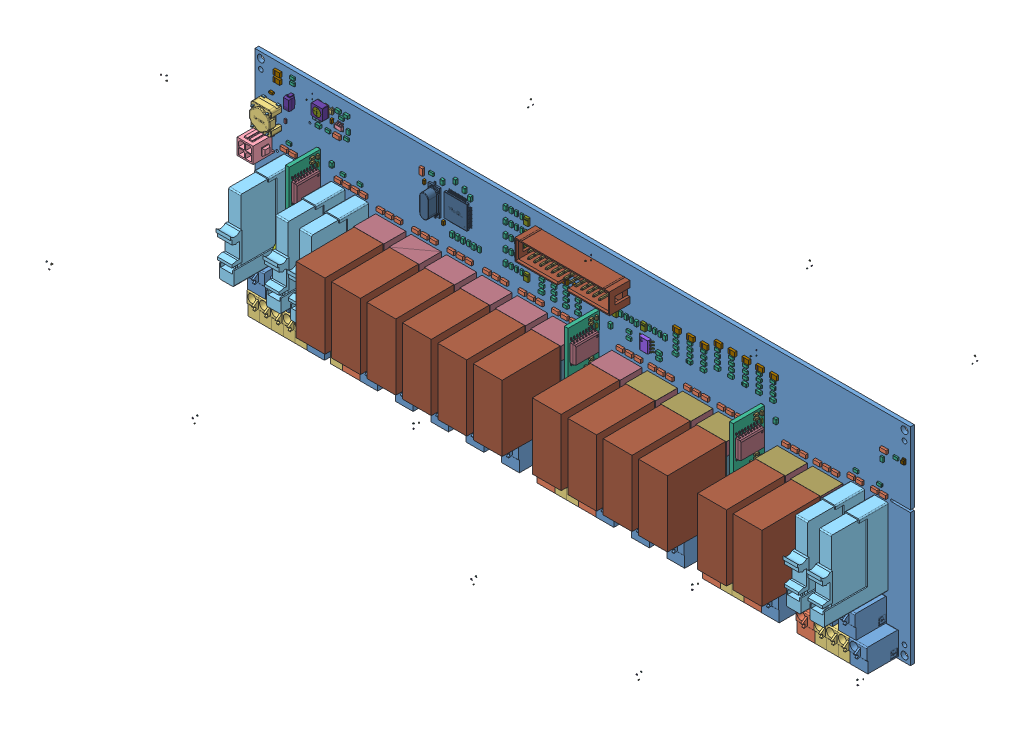
SolidWorks assembly _SC940D, configuration Default. Lengths in mm.
Overall size (350.55 148.8 148.76).
1323 component instances, 58 part files, 0 mates.
Components (placement in the parent):
- Board-1: Board [Default] at (0 0 -1.6703) size (281.94 89 1.67)
- D19-1: D19 [Default] at origin size (14.37 27.55 23.48)
  - SW3dPS-transistor_SOT233_4-1: SW3dPS-transistor_SOT233_4 [Default] at (10.8838 24.6832 -21.9) x (-1 0 0) z (0 1 0) size (2.9 1.1 1.6)
  - SW3dPS-transistor_SOT233_5-1: SW3dPS-transistor_SOT233_5 [Default] at (0.0109 0.0247 -0.0219) x (-1 0 0) z (0 1 0) size (2.18 2.18 2.18)
  - SW3dPS-transistor_SOT233_6-1: SW3dPS-transistor_SOT233_6 [Default] at (0 0 0) x (-1 0 0) z (0 1 0) size (2.18 2.18 2.18)
  - SW3dPS-transistor_SOT233_7-1: SW3dPS-transistor_SOT233_7 [Default] x (-1 0 0) z (0 1 0) size (2.18 2.18 2.18)
- U5-1: U5 [Default] at origin size (27.38 148.76 148.76)
  - SC943-0C_20-12-2012-1: SC943-0C_20-12-2012 [Default] at (142.3952 27.9566 3.7281) x (0 1 0.000663) z (1 0 0) size (148.66 148.66 27.38)
    - Board_1-1: Board_1 [Default] at (0 0 -1.6167) size (43.5 16.8 1.62)
    - R15-1: R15 [Default] at origin size (1.6 0.8 0.55)
      - RESC1608X84N_1-1: RESC1608X84N_1 [Default] at (-0.0001 1.9049 0) x (-1 0 0) z (0 1 0) size (1.6 0.55 0.8)
    - R11-1: R11 [Default] at origin size (2 1.2 0.7)
      - RESC2012X70N_1-1: RESC2012X70N_1 [Default] at (-3.6513 -0.4763 0) x (-1 0 0) z (0 1 0) size (2 0.7 1.2)
    - R7-1: R7 [Default] at origin size (2 1.2 0.7)
      - RESC2012X70N_1-1: RESC2012X70N_1 [Default] at (-5.2388 1.5874 0) x (-1 0 0) z (0 1 0) size (2 0.7 1.2)
    - D3-1: D3 [Default] at origin size (2.6 5.2 2.43)
      - SW3dPS-DO-214AC_SMA-1: SW3dPS-DO-214AC_SMA [Default] at (-1.4287 0.3175 -2.9167) x (1 0 0) z (0 0 -1) size (2.6 5.2 2.43)
    - T4-1: T4 [Default] at origin size (6.54 9.94 2.42)
      - SW3dPS-DPAK-1-1: SW3dPS-DPAK-1 [Default] at (10.9238 2.2758 -2.8167) x (1 0 0) z (0 1 0) size (6.54 2.42 9.94)
    - T3-1: T3 [Default] at origin size (6.54 9.94 2.42)
      - SW3dPS-DPAK-1-1: SW3dPS-DPAK-1 [Default] at (-10.3487 2.2758 -2.8167) x (1 0 0) z (0 1 0) size (6.54 2.42 9.94)
    - D5-1: D5 [Default] at origin size (2.6 5.2 2.43)
      - SW3dPS-DO-214AC_SMA-1: SW3dPS-DO-214AC_SMA [Default] at (2.0638 0.3175 -2.9167) x (1 0 0) z (0 0 -1) size (2.6 5.2 2.43)
    - D4-1: D4 [Default] at origin size (2.6 5.2 2.43)
      - SW3dPS-DO-214AC_SMA-1: SW3dPS-DO-214AC_SMA [Default] at (5.2388 0.3175 -2.9167) x (1 0 0) z (0 0 -1) size (2.6 5.2 2.43)
    - D2-1: D2 [Default] at origin size (2.6 5.2 2.43)
      - SW3dPS-DO-214AC_SMA-1: SW3dPS-DO-214AC_SMA [Default] at (-4.6037 0.3175 -2.9167) x (1 0 0) z (0 0 -1) size (2.6 5.2 2.43)
    - R25-1: R25 [Default] at origin size (3.2 1.6 0.84)
      - RESC3216X84N-1: RESC3216X84N [Default] at (-2.0851 5.5563 -1.6167) x (-1 0 0) z (0 -1 0) size (3.2 0.84 1.6)
    - R26-1: R26 [Default] at origin size (3.2 1.6 0.84)
      - RESC3216X84N-1: RESC3216X84N [Default] at (2.6989 5.5562 -1.6167) x (1 0 0) z (0 1 0) size (3.2 0.84 1.6)
    - C6-1: C6 [Default] at origin size (0.8 1.6 0.9)
      - User_Library-CAPC1608X09_1-1: User_Library-CAPC1608X09_1 [Default] at (10.0013 0.1587 0) x (0 -1 0) z (0 0 1) size (1.6 0.8 0.9)
    - C7-1: C7 [Default] at origin size (0.8 1.6 0.9)
      - User_Library-CAPC1608X09_1-1: User_Library-CAPC1608X09_1 [Default] at (27.7813 0.1587 0) x (0 -1 0) z (0 0 1) size (1.6 0.8 0.9)
    - C8-1: C8 [Default] at origin size (0.8 1.6 0.9)
      - User_Library-CAPC1608X09_1-1: User_Library-CAPC1608X09_1 [Default] at (26.1938 0.1587 0) x (0 -1 0) z (0 0 1) size (1.6 0.8 0.9)
    - C9-1: C9 [Default] at origin size (1.6 0.8 0.9)
      - User_Library-CAPC1608X09_1-1: User_Library-CAPC1608X09_1 [Default] at (7.7788 2.3813 0) size (1.6 0.8 0.9)
    - L1-1: L1 [Default] at origin size (1.6 0.8 0.9)
      - User_Library-CAPC1608X09_1-1: User_Library-CAPC1608X09_1 [Default] at (10.7949 -2.0638 0) x (-1 0 0) z (0 0 1) size (1.6 0.8 0.9)
    - L2-1: L2 [Default] at origin size (1.6 0.8 0.9)
      - User_Library-CAPC1608X09_1-1: User_Library-CAPC1608X09_1 [Default] at (27.1463 -2.2224 0) size (1.6 0.8 0.9)
    - L3-1: L3 [Default] at origin size (1.6 0.8 0.9)
      - User_Library-CAPC1608X09_1-1: User_Library-CAPC1608X09_1 [Default] at (10.7949 2.3812 0) x (-1 0 0) z (0 0 1) size (1.6 0.8 0.9)
    - U1-1: U1 [Default] at origin size (10.3 10.3 2.65)
      - SW3dPS-SOIC16-300-1: SW3dPS-SOIC16-300 [Default] at (19.685 3.9689 0) x (0 1 0) z (0 0 1) size (10.3 10.3 2.65)
    - R2-1: R2 [Default] at origin size (2 1.2 0.7)
      - RESC2012X70N_1-1: RESC2012X70N_1 [Default] at (-8.7312 1.9051 0) x (1 0 0) z (0 -1 0) size (2 0.7 1.2)
    - C4-1: C4 [Default] at origin size (0.8 1.6 0.9)
      - User_Library-CAPC1608X09_1-1: User_Library-CAPC1608X09_1 [Default] at (-13.0176 7.6201 0) x (0 1 0) z (0 0 1) size (1.6 0.8 0.9)
    - T6-1: T6 [Default] at origin size (36.29 81.18 23.48)
      - SW3dPS-transistor_SOT233-1: SW3dPS-transistor_SOT233 [Default] at (-33.4193 77.6987 -21.9) x (0 1 0) z (1 0 0) size (2.9 1.1 1.6)
      - SW3dPS-transistor_SOT233_1-1: SW3dPS-transistor_SOT233_1 [Default] at (-0.0334 0.0777 -0.0219) x (0 1 0) z (1 0 0) size (2.18 2.18 2.18)
      - SW3dPS-transistor_SOT233_2-1: SW3dPS-transistor_SOT233_2 [Default] at (0 0.0001 0) x (0 1 0) z (1 0 0) size (2.18 2.18 2.18)
      - SW3dPS-transistor_SOT233_3-1: SW3dPS-transistor_SOT233_3 [Default] x (0 1 0) z (1 0 0) size (2.18 2.18 2.18)
    - U2-1: U2 [Default] at origin size (6.2 5 1.75)
      - User_Library-SOIC-8-150-1: User_Library-SOIC-8-150 [Default] at (6.9849 6.3501 1) x (0 -1 0) z (-1 0 0) size (5 1.75 6.2)
        - User_Library-SOIC-8-150_pin_SOIC_SO-150_1_1-1: User_Library-SOIC-8-150_pin_SOIC_SO-150_1_1 [Default] at (0.6 0 -2) x (-1 0 0) z (0 0 -1) size (0.4 1.1 1.1)
        - User_Library-SOIC-8-150_pin_SOIC_SO-150_1_1-2: User_Library-SOIC-8-150_pin_SOIC_SO-150_1_1 [Default] at (-0.67 0 -2) x (-1 0 0) z (0 0 -1) size (0.4 1.1 1.1)
        - User_Library-SOIC-8-150_pin_SOIC_SO-150_1_1-3: User_Library-SOIC-8-150_pin_SOIC_SO-150_1_1 [Default] at (-1.94 0 2) size (0.4 1.1 1.1)
        - User_Library-SOIC-8-150_pin_SOIC_SO-150_1_1-4: User_Library-SOIC-8-150_pin_SOIC_SO-150_1_1 [Default] at (-0.67 0 2) size (0.4 1.1 1.1)
        - User_Library-SOIC-8-150_pin_SOIC_SO-150_1_1-5: User_Library-SOIC-8-150_pin_SOIC_SO-150_1_1 [Default] at (-1.94 0 -2) x (-1 0 0) z (0 0 -1) size (0.4 1.1 1.1)
        - User_Library-SOIC-8-150_pin_SOIC_SO-150_1_1-6: User_Library-SOIC-8-150_pin_SOIC_SO-150_1_1 [Default] at (1.87 0 2) size (0.4 1.1 1.1)
        - User_Library-SOIC-8-150_SOIC_150_SOIC_5X4_1_1-1: User_Library-SOIC-8-150_SOIC_150_SOIC_5X4_1_1 [Default] at origin size (5 1.5 4)
        - User_Library-SOIC-8-150_pin_SOIC_SO-150_1_1-7: User_Library-SOIC-8-150_pin_SOIC_SO-150_1_1 [Default] at (0.6 0 2) size (0.4 1.1 1.1)
        - User_Library-SOIC-8-150_pin_SOIC_SO-150_1_1-8: User_Library-SOIC-8-150_pin_SOIC_SO-150_1_1 [Default] at (1.87 0 -2) x (-1 0 0) z (0 0 -1) size (0.4 1.1 1.1)
    - R16-1: R16 [Default] at origin size (1.2 2 0.7)
      - RESC2012X70N_1-1: RESC2012X70N_1 [Default] at (-3.1751 7.3026 0) x (0 1 0) z (1 0 0) size (2 0.7 1.2)
    - R12-1: R12 [Default] at origin size (1.2 2 0.7)
      - RESC2012X70N_1-1: RESC2012X70N_1 [Default] at (2.2226 -1.2701 0) x (0 -1 0) z (-1 0 0) size (2 0.7 1.2)
    - R9-1: R9 [Default] at origin size (1.6 0.8 0.55)
      - RESC1608X84N_1-1: RESC1608X84N_1 [Default] at (1.5874 5.5562 0) x (-1 0 0) z (0 1 0) size (1.6 0.55 0.8)
    - R8-1: R8 [Default] at origin size (2 1.2 0.7)
      - RESC2012X70N_1-1: RESC2012X70N_1 [Default] at (5.0801 -1.9049 0) x (1 0 0) z (0 -1 0) size (2 0.7 1.2)
    - C5-1: C5 [Default] at origin size (0.8 1.6 0.9)
      - User_Library-CAPC1608X09_1-1: User_Library-CAPC1608X09_1 [Default] at (11.5888 0.1587 0) x (0 -1 0) z (0 0 1) size (1.6 0.8 0.9)
    - C3-1: C3 [Default] at origin size (0.8 1.6 0.9)
      - User_Library-CAPC1608X09_1-1: User_Library-CAPC1608X09_1 [Default] at (8.4138 0.1587 0) x (0 -1 0) z (0 0 1) size (1.6 0.8 0.9)
    - C2-1: C2 [Default] at origin size (0.8 1.6 0.9)
      - User_Library-CAPC1608X09_1-1: User_Library-CAPC1608X09_1 [Default] at (13.1763 0.1587 0) x (0 -1 0) z (0 0 1) size (1.6 0.8 0.9)
    - R17-1: R17 [Default] at origin size (0.8 1.6 0.55)
      - RESC1608X84N_1-1: RESC1608X84N_1 [Default] at (-1.2701 7.6201 0) x (0 1 0) z (1 0 0) size (1.6 0.55 0.8)
    - R18-1: R18 [Default] at origin size (1.6 0.8 0.55)
      - RESC1608X84N_1-1: RESC1608X84N_1 [Default] at (-6.9851 8.2549 0) x (-1 0 0) z (0 1 0) size (1.6 0.55 0.8)
    - T5-1: T5 [Default] at origin size (82.76 20.1 23.48)
      - SW3dPS-transistor_SOT233-1: SW3dPS-transistor_SOT233 [Default] at (-79.2862 -17.2268 -21.9) x (-1 0 0) z (0 1 0) size (2.9 1.1 1.6)
      - SW3dPS-transistor_SOT233_1-1: SW3dPS-transistor_SOT233_1 [Default] at (-0.0793 -0.0172 -0.0219) x (-1 0 0) z (0 1 0) size (2.18 2.18 2.18)
      - SW3dPS-transistor_SOT233_2-1: SW3dPS-transistor_SOT233_2 [Default] at (-0.0001 0 0) x (-1 0 0) z (0 1 0) size (2.18 2.18 2.18)
      - SW3dPS-transistor_SOT233_3-1: SW3dPS-transistor_SOT233_3 [Default] x (-1 0 0) z (0 1 0) size (2.18 2.18 2.18)
    - T7-1: T7 [Default] at origin size (73.54 29.78 23.48)
      - SW3dPS-transistor_SOT233-1: SW3dPS-transistor_SOT233 [Default] at (70.0609 26.9106 -21.9) x (1 0 0) z (0 -1 0) size (2.9 1.1 1.6)
      - SW3dPS-transistor_SOT233_1-1: SW3dPS-transistor_SOT233_1 [Default] at (0.0701 0.0269 -0.0219) x (1 0 0) z (0 -1 0) size (2.18 2.18 2.18)
      - SW3dPS-transistor_SOT233_2-1: SW3dPS-transistor_SOT233_2 [Default] at (0.0001 0 0) x (1 0 0) z (0 -1 0) size (2.18 2.18 2.18)
      - SW3dPS-transistor_SOT233_3-1: SW3dPS-transistor_SOT233_3 [Default] x (1 0 0) z (0 -1 0) size (2.18 2.18 2.18)
    - C1-1: C1 [Default] at origin size (1.6 0.8 0.9)
      - User_Library-CAPC1608X09_1-1: User_Library-CAPC1608X09_1 [Default] at (27.1462 -1.9049 -1.6167) x (-1 0 0) z (0 0 -1) size (1.6 0.8 0.9)
    - R19-1: R19 [Default] at origin size (1.6 0.8 0.55)
      - RESC1608X84N_1-1: RESC1608X84N_1 [Default] at (-10.7949 8.2551 0) x (1 0 0) z (0 -1 0) size (1.6 0.55 0.8)
    - R1-1: R1 [Default] at origin size (1.6 0.8 0.55)
      - RESC1608X84N_1-1: RESC1608X84N_1 [Default] at (24.1301 -2.2224 0) x (1 0 0) z (0 -1 0) size (1.6 0.55 0.8)
    - D1-1: D1 [Default] at origin size (80.06 27.08 23.48)
      - SW3dPS-transistor_SOT233-1: SW3dPS-transistor_SOT233 [Default] at (76.5874 24.2118 -21.9) x (1 0 0) z (0 -1 0) size (2.9 1.1 1.6)
      - SW3dPS-transistor_SOT233_1-1: SW3dPS-transistor_SOT233_1 [Default] at (0.0766 0.0242 -0.0219) x (1 0 0) z (0 -1 0) size (2.18 2.18 2.18)
      - SW3dPS-transistor_SOT233_2-1: SW3dPS-transistor_SOT233_2 [Default] at (0.0001 0 0) x (1 0 0) z (0 -1 0) size (2.18 2.18 2.18)
      - SW3dPS-transistor_SOT233_3-1: SW3dPS-transistor_SOT233_3 [Default] x (1 0 0) z (0 -1 0) size (2.18 2.18 2.18)
    - D6-1: D6 [Default] at origin size (13.75 77.05 23.48)
      - SW3dPS-transistor_SOT233-1: SW3dPS-transistor_SOT233 [Default] at (10.8768 -73.5712 -21.9) x (0 -1 0) z (-1 0 0) size (2.9 1.1 1.6)
      - SW3dPS-transistor_SOT233_1-1: SW3dPS-transistor_SOT233_1 [Default] at (0.0109 -0.0736 -0.0219) x (0 -1 0) z (-1 0 0) size (2.18 2.18 2.18)
      - SW3dPS-transistor_SOT233_2-1: SW3dPS-transistor_SOT233_2 [Default] at (0 -0.0001 0) x (0 -1 0) z (-1 0 0) size (2.18 2.18 2.18)
      - SW3dPS-transistor_SOT233_3-1: SW3dPS-transistor_SOT233_3 [Default] x (0 -1 0) z (-1 0 0) size (2.18 2.18 2.18)
    - D7-1: D7 [Default] at origin size (17.72 77.05 23.48)
      - SW3dPS-transistor_SOT233-1: SW3dPS-transistor_SOT233 [Default] at (14.8456 -73.5712 -21.9) x (0 -1 0) z (-1 0 0) size (2.9 1.1 1.6)
      - SW3dPS-transistor_SOT233_1-1: SW3dPS-transistor_SOT233_1 [Default] at (0.0148 -0.0736 -0.0219) x (0 -1 0) z (-1 0 0) size (2.18 2.18 2.18)
      - SW3dPS-transistor_SOT233_2-1: SW3dPS-transistor_SOT233_2 [Default] at (0 -0.0001 0) x (0 -1 0) z (-1 0 0) size (2.18 2.18 2.18)
      - SW3dPS-transistor_SOT233_3-1: SW3dPS-transistor_SOT233_3 [Default] x (0 -1 0) z (-1 0 0) size (2.18 2.18 2.18)
    - R3-1: R3 [Default] at origin size (2 1.2 0.7)
      - RESC2012X70N_1-1: RESC2012X70N_1 [Default] at (-12.2237 1.9051 0) x (1 0 0) z (0 -1 0) size (2 0.7 1.2)
- L3_1-1: L3_1 [Default] at origin size (8.76 10 6)
  - STEP-744272102-rev1_RGB8421504-1: STEP-744272102-rev1_RGB8421504 [Default] at (1.7783 60.1986 0.3127) x (-1 0 0) z (0 0 1) size (8.76 10 6)
    - Base_5-1: Base_5 [Default] at origin size (5 6.5 2.6)
    - Base_6-1: Base_6 [Default] at origin size (8.76 10 5.3)
    - Base_1-1: Base_1 [Default] at origin size (3.01 7.71 4.33)
    - Contact-1: Contact [Default] at (-3.11 -3.66 -0.3) x (-1 0 0) z (0 0 -1) size (1.2 1.83 6)
    - Contact-2: Contact [Default] at (3.11 -3.66 -0.3) x (-1 0 0) z (0 0 -1) size (1.2 1.83 6)
    - Contact-3: Contact [Default] at (-3.11 3.66 -0.3) x (1 0 0) z (0 0 -1) size (1.2 1.83 6)
    - Contact-4: Contact [Default] at (3.11 3.66 -0.3) x (1 0 0) z (0 0 -1) size (1.2 1.83 6)
- C39-1: C39 [Default] at origin size (2 1.25 1)
  - User_Library-CAPC2013X10-1: User_Library-CAPC2013X10 [Default] at (168.5924 52.2287 0) x (-1 0 0) z (0 0 1) size (2 1.25 1)
- C38-1: C38 [Default] at origin size (2 1.25 1)
  - User_Library-CAPC2013X10-1: User_Library-CAPC2013X10 [Default] at (168.5926 54.2926 0) x (1 0 0) z (0 0 1) size (2 1.25 1)
- VR1-1: VR1 [Default] at origin size (3.59 9 34)
  - WE-VD_7_mm-1: WE-VD_7_mm [Default] at (15.5576 20.1613 9) x (0 1 0) z (0 0 1) size (9 3.59 34)
- D38-1: D38 [Default] at origin size (2.9 1.9 0.99)
  - 905269800-1: 905269800 [Default] at (187.579 66.802 0.95) size (0.25 1.78 0.04)
    - Extruded-1: Extruded [Default] at origin size (0.25 1.78 0.04)
  - 905269392-1: 905269392 [Default] at (188.214 66.802 0) size (2.9 1.9 0.98)
    - Extruded_1-1: Extruded_1 [Default] at origin size (2.9 1.9 0.98)
- U4-1: U4 [Default] at origin size (12.02 12.02 1.1)
  - User_Library-TQFP64-1: User_Library-TQFP64 [Default] at (81.6561 63.8895 0) x (-1 0 0) z (0 0 1) size (12.02 12.02 1.1)
- K13-1: K13 [Default] at origin size (13 30.3 34.5)
  - relais_40_61_8_006_0000-1: relais_40_61_8_006_0000 [Default] at (200.025 15.6766 9.5) x (0 1 0) z (1 0 0) size (29 30 12.4)
  - 1151724792-1: 1151724792 [Default] at (200.025 21.78 0) size (13 14.8 9.5)
    - Extruded_2-1: Extruded_2 [Default] at origin size (13 14.8 9.5)
  - 1151724928-1: 1151724928 [Default] at (200.025 41.93 0) size (13 5.5 9.5)
    - Extruded_3-1: Extruded_3 [Default] at origin size (13 5.5 9.5)
  - 1151725064-1: 1151725064 [Default] at (200.025 34.18 5) size (13 10 4.5)
    - Extruded_4-1: Extruded_4 [Default] at origin size (13 10 4.5)
- SUP_K13-1: SUP_K13 [Default] at origin size (13 30.3 9.5)
  - 1151724792-1: 1151724792 [Default] at (200.025 37.325 0) size (13 14.8 9.5)
    - Extruded_2-1: Extruded_2 [Default] at origin size (13 14.8 9.5)
  - 1151725064-1: 1151725064 [Default] at (200.025 24.925 5) size (13 10 4.5)
    - Extruded_4-1: Extruded_4 [Default] at origin size (13 10 4.5)
  - 1151724928-1: 1151724928 [Default] at (200.025 17.175 0) size (13 5.5 9.5)
    - Extruded_3-1: Extruded_3 [Default] at origin size (13 5.5 9.5)
- SUP_K12-1: SUP_K12 [Default] at origin size (13 30.3 9.5)
  - 1151724792-1: 1151724792 [Default] at (184.785 37.325 0) size (13 14.8 9.5)
    - Extruded_2-1: Extruded_2 [Default] at origin size (13 14.8 9.5)
  - 1151725064-1: 1151725064 [Default] at (184.785 24.925 5) size (13 10 4.5)
    - Extruded_4-1: Extruded_4 [Default] at origin size (13 10 4.5)
  - 1151724928-1: 1151724928 [Default] at (184.785 17.175 0) size (13 5.5 9.5)
    - Extruded_3-1: Extruded_3 [Default] at origin size (13 5.5 9.5)
- K12-1: K12 [Default] at origin size (13 30.3 34.5)
  - relais_40_61_8_006_0000-1: relais_40_61_8_006_0000 [Default] at (184.785 15.6766 9.5) x (0 1 0) z (1 0 0) size (29 30 12.4)
  - 1151724792-1: 1151724792 [Default] at (184.785 21.78 0) size (13 14.8 9.5)
    - Extruded_2-1: Extruded_2 [Default] at origin size (13 14.8 9.5)
  - 1151724928-1: 1151724928 [Default] at (184.785 41.93 0) size (13 5.5 9.5)
    - Extruded_3-1: Extruded_3 [Default] at origin size (13 5.5 9.5)
  - 1151725064-1: 1151725064 [Default] at (184.785 34.18 5) size (13 10 4.5)
    - Extruded_4-1: Extruded_4 [Default] at origin size (13 10 4.5)
- C34-1: C34 [Default] at origin size (1.25 2 1)
  - User_Library-CAPC2013X10-1: User_Library-CAPC2013X10 [Default] at (218.8159 54.1717 0) x (0 -1 0) z (0 0 1) size (2 1.25 1)
- C27-1: C27 [Default] at origin size (1.25 2 1)
  - User_Library-CAPC2013X10-1: User_Library-CAPC2013X10 [Default] at (147.6959 54.1717 0) x (0 -1 0) z (0 0 1) size (2 1.25 1)
- C5_1-1: C5_1 [Default] at origin size (1.25 2 1)
  - User_Library-CAPC2013X10-1: User_Library-CAPC2013X10 [Default] at (27.8194 54.1717 0) x (0 -1 0) z (0 0 1) size (2 1.25 1)
- VR2-1: VR2 [Default] at origin size (3.59 9 34)
  - WE-VD_7_mm-1: WE-VD_7_mm [Default] at (133.9849 8.3979 9) x (0 -1 0) z (0 0 1) size (9 3.59 34)
- D28-1: D28 [Default] at origin size (1.9 2.9 0.99)
  - 1151710512-1: 1151710512 [Default] at (162.052 61.595 0.95) size (1.78 0.25 0.04)
    - Extruded_5-1: Extruded_5 [Default] at origin size (1.78 0.25 0.04)
  - 1151710376-1: 1151710376 [Default] at (162.052 60.96 0) size (1.9 2.9 0.98)
    - Extruded_6-1: Extruded_6 [Default] at origin size (1.9 2.9 0.98)
- VR3-1: VR3 [Default] at origin size (3.59 9 34)
  - WE-VD_7_mm-1: WE-VD_7_mm [Default] at (205.1049 8.3979 9) x (0 -1 0) z (0 0 1) size (9 3.59 34)
- D2_1-1: D2_1 [Default] at origin size (2.9 1.9 0.99)
  - 905269800-1: 905269800 [Default] at (3.8418 73.803 0.95) size (0.25 1.78 0.04)
    - Extruded-1: Extruded [Default] at origin size (0.25 1.78 0.04)
  - 905269392-1: 905269392 [Default] at (4.4767 73.803 0) size (2.9 1.9 0.98)
    - Extruded_1-1: Extruded_1 [Default] at origin size (2.9 1.9 0.98)
- D1_1-1: D1_1 [Default] at origin size (2.9 1.9 0.99)
  - 905269800-1: 905269800 [Default] at (3.8418 76.5017 0.95) size (0.25 1.78 0.04)
    - Extruded-1: Extruded [Default] at origin size (0.25 1.78 0.04)
  - 905269392-1: 905269392 [Default] at (4.4767 76.5017 0) size (2.9 1.9 0.98)
    - Extruded_1-1: Extruded_1 [Default] at origin size (2.9 1.9 0.98)
- D41-1: D41 [Default] at origin size (2.9 1.9 0.99)
  - 905269800-1: 905269800 [Default] at (193.548 70.358 0.95) size (0.25 1.78 0.04)
    - Extruded-1: Extruded [Default] at origin size (0.25 1.78 0.04)
  - 905269392-1: 905269392 [Default] at (194.183 70.358 0) size (2.9 1.9 0.98)
    - Extruded_1-1: Extruded_1 [Default] at origin size (2.9 1.9 0.98)
- D40-1: D40 [Default] at origin size (2.9 1.9 0.99)
  - 905269800-1: 905269800 [Default] at (199.517 70.358 0.95) size (0.25 1.78 0.04)
    - Extruded-1: Extruded [Default] at origin size (0.25 1.78 0.04)
  - 905269392-1: 905269392 [Default] at (200.152 70.358 0) size (2.9 1.9 0.98)
    - Extruded_1-1: Extruded_1 [Default] at origin size (2.9 1.9 0.98)
- D36-1: D36 [Default] at origin size (2.9 1.9 0.99)
  - 905269800-1: 905269800 [Default] at (205.486 70.358 0.95) size (0.25 1.78 0.04)
    - Extruded-1: Extruded [Default] at origin size (0.25 1.78 0.04)
  - 905269392-1: 905269392 [Default] at (206.121 70.358 0) size (2.9 1.9 0.98)
    - Extruded_1-1: Extruded_1 [Default] at origin size (2.9 1.9 0.98)
- D35-1: D35 [Default] at origin size (2.9 1.9 0.99)
  - 905269800-1: 905269800 [Default] at (181.61 66.802 0.95) size (0.25 1.78 0.04)
    - Extruded-1: Extruded [Default] at origin size (0.25 1.78 0.04)
  - 905269392-1: 905269392 [Default] at (182.245 66.802 0) size (2.9 1.9 0.98)
    - Extruded_1-1: Extruded_1 [Default] at origin size (2.9 1.9 0.98)
- D33-1: D33 [Default] at origin size (2.9 1.9 0.99)
  - 905269800-1: 905269800 [Default] at (211.455 70.358 0.95) size (0.25 1.78 0.04)
    - Extruded-1: Extruded [Default] at origin size (0.25 1.78 0.04)
  - 905269392-1: 905269392 [Default] at (212.09 70.358 0) size (2.9 1.9 0.98)
    - Extruded_1-1: Extruded_1 [Default] at origin size (2.9 1.9 0.98)
- D32-1: D32 [Default] at origin size (2.9 1.9 0.99)
  - 905269800-1: 905269800 [Default] at (217.424 70.358 0.95) size (0.25 1.78 0.04)
    - Extruded-1: Extruded [Default] at origin size (0.25 1.78 0.04)
  - 905269392-1: 905269392 [Default] at (218.059 70.358 0) size (2.9 1.9 0.98)
    - Extruded_1-1: Extruded_1 [Default] at origin size (2.9 1.9 0.98)
- D30-1: D30 [Default] at origin size (2.9 1.9 0.99)
  - 905269800-1: 905269800 [Default] at (175.641 66.802 0.95) size (0.25 1.78 0.04)
    - Extruded-1: Extruded [Default] at origin size (0.25 1.78 0.04)
  - 905269392-1: 905269392 [Default] at (176.276 66.802 0) size (2.9 1.9 0.98)
    - Extruded_1-1: Extruded_1 [Default] at origin size (2.9 1.9 0.98)
- D26-1: D26 [Default] at origin size (1.9 2.9 0.99)
  - 1151710512-1: 1151710512 [Default] at (149.733 60.706 0.95) size (1.78 0.25 0.04)
    - Extruded_5-1: Extruded_5 [Default] at origin size (1.78 0.25 0.04)
  - 1151710376-1: 1151710376 [Default] at (149.733 60.071 0) size (1.9 2.9 0.98)
    - Extruded_6-1: Extruded_6 [Default] at origin size (1.9 2.9 0.98)
- D22-1: D22 [Default] at origin size (1.9 2.9 0.99)
  - 1151710512-1: 1151710512 [Default] at (137.414 60.706 0.95) size (1.78 0.25 0.04)
    - Extruded_5-1: Extruded_5 [Default] at origin size (1.78 0.25 0.04)
  - 1151710376-1: 1151710376 [Default] at (137.414 60.071 0) size (1.9 2.9 0.98)
    - Extruded_6-1: Extruded_6 [Default] at origin size (1.9 2.9 0.98)
- D20-1: D20 [Default] at origin size (2.9 1.9 0.99)
  - 905269800-1: 905269800 [Default] at (133.858 60.96 0.95) size (0.25 1.78 0.04)
    - Extruded-1: Extruded [Default] at origin size (0.25 1.78 0.04)
  - 905269392-1: 905269392 [Default] at (133.223 60.96 0) size (2.9 1.9 0.98)
    - Extruded_1-1: Extruded_1 [Default] at origin size (2.9 1.9 0.98)
- D17-1: D17 [Default] at origin size (2.9 1.9 0.99)
  - 905269800-1: 905269800 [Default] at (123.444 60.96 0.95) size (0.25 1.78 0.04)
    - Extruded-1: Extruded [Default] at origin size (0.25 1.78 0.04)
  - 905269392-1: 905269392 [Default] at (122.809 60.96 0) size (2.9 1.9 0.98)
    - Extruded_1-1: Extruded_1 [Default] at origin size (2.9 1.9 0.98)
- D14-1: D14 [Default] at origin size (2.9 1.9 0.99)
  - 905269800-1: 905269800 [Default] at (128.651 60.96 0.95) size (0.25 1.78 0.04)
    - Extruded-1: Extruded [Default] at origin size (0.25 1.78 0.04)
  - 905269392-1: 905269392 [Default] at (128.016 60.96 0) size (2.9 1.9 0.98)
    - Extruded_1-1: Extruded_1 [Default] at origin size (2.9 1.9 0.98)
- D12-1: D12 [Default] at origin size (2.9 1.9 0.99)
  - 905269800-1: 905269800 [Default] at (118.237 60.96 0.95) size (0.25 1.78 0.04)
    - Extruded-1: Extruded [Default] at origin size (0.25 1.78 0.04)
  - 905269392-1: 905269392 [Default] at (117.602 60.96 0) size (2.9 1.9 0.98)
    - Extruded_1-1: Extruded_1 [Default] at origin size (2.9 1.9 0.98)
- D21-1: D21 [Default] at origin size (1.9 2.9 0.99)
  - 1151710512-1: 1151710512 [Default] at (111.76 60.071 0.95) size (1.78 0.25 0.04)
    - Extruded_5-1: Extruded_5 [Default] at origin size (1.78 0.25 0.04)
  - 1151710376-1: 1151710376 [Default] at (111.76 59.436 0) size (1.9 2.9 0.98)
    - Extruded_6-1: Extruded_6 [Default] at origin size (1.9 2.9 0.98)
- D18-1: D18 [Default] at origin size (1.9 2.9 0.99)
  - 1151710512-1: 1151710512 [Default] at (111.76 54.864 0.95) size (1.78 0.25 0.04)
    - Extruded_5-1: Extruded_5 [Default] at origin size (1.78 0.25 0.04)
  - 1151710376-1: 1151710376 [Default] at (111.76 54.229 0) size (1.9 2.9 0.98)
    - Extruded_6-1: Extruded_6 [Default] at origin size (1.9 2.9 0.98)
- D16-1: D16 [Default] at origin size (1.9 2.9 0.99)
  - 1151710512-1: 1151710512 [Default] at (111.76 75.692 0.95) size (1.78 0.25 0.04)
    - Extruded_5-1: Extruded_5 [Default] at origin size (1.78 0.25 0.04)
  - 1151710376-1: 1151710376 [Default] at (111.76 75.057 0) size (1.9 2.9 0.98)
    - Extruded_6-1: Extruded_6 [Default] at origin size (1.9 2.9 0.98)
- D13-1: D13 [Default] at origin size (1.9 2.9 0.99)
  - 1151710512-1: 1151710512 [Default] at (111.76 65.278 0.95) size (1.78 0.25 0.04)
    - Extruded_5-1: Extruded_5 [Default] at origin size (1.78 0.25 0.04)
  - 1151710376-1: 1151710376 [Default] at (111.76 64.643 0) size (1.9 2.9 0.98)
    - Extruded_6-1: Extruded_6 [Default] at origin size (1.9 2.9 0.98)
- D10-1: D10 [Default] at origin size (1.9 2.9 0.99)
  - 1151710512-1: 1151710512 [Default] at (111.76 70.485 0.95) size (1.78 0.25 0.04)
    - Extruded_5-1: Extruded_5 [Default] at origin size (1.78 0.25 0.04)
  - 1151710376-1: 1151710376 [Default] at (111.76 69.85 0) size (1.9 2.9 0.98)
    - Extruded_6-1: Extruded_6 [Default] at origin size (1.9 2.9 0.98)
- C6_1-1: C6_1 [Default] at origin size (1.25 2 1)
  - User_Library-CAPC2013X10-1: User_Library-CAPC2013X10 [Default] at (102.616 70.3579 0) x (0 -1 0) z (0 0 1) size (2 1.25 1)
- C8_1-1: C8_1 [Default] at origin size (1.25 2 1)
  - User_Library-CAPC2013X10-1: User_Library-CAPC2013X10 [Default] at (102.616 65.1509 0) x (0 -1 0) z (0 0 1) size (2 1.25 1)
- C10-1: C10 [Default] at origin size (1.25 2 1)
  - User_Library-CAPC2013X10-1: User_Library-CAPC2013X10 [Default] at (102.616 75.5649 0) x (0 -1 0) z (0 0 1) size (2 1.25 1)
- C12-1: C12 [Default] at origin size (1.25 2 1)
  - User_Library-CAPC2013X10-1: User_Library-CAPC2013X10 [Default] at (102.616 54.7369 0) x (0 -1 0) z (0 0 1) size (2 1.25 1)
- C11-1: C11 [Default] at origin size (2 1.25 1)
  - User_Library-CAPC2013X10-1: User_Library-CAPC2013X10 [Default] at (123.3169 51.816 0) x (-1 0 0) z (0 0 1) size (2 1.25 1)
- C28-1: C28 [Default] at origin size (1.25 2 1)
  - User_Library-CAPC2013X10-1: User_Library-CAPC2013X10 [Default] at (171.196 61.4679 0) x (0 -1 0) z (0 0 1) size (2 1.25 1)
- C14-1: C14 [Default] at origin size (1.25 2 1)
  - User_Library-CAPC2013X10-1: User_Library-CAPC2013X10 [Default] at (102.616 59.9439 0) x (0 -1 0) z (0 0 1) size (2 1.25 1)
- C7_1-1: C7_1 [Default] at origin size (2 1.25 1)
  - User_Library-CAPC2013X10-1: User_Library-CAPC2013X10 [Default] at (118.1099 51.816 0) x (-1 0 0) z (0 0 1) size (2 1.25 1)
- C9_1-1: C9_1 [Default] at origin size (2 1.25 1)
  - User_Library-CAPC2013X10-1: User_Library-CAPC2013X10 [Default] at (128.5239 51.816 0) x (-1 0 0) z (0 0 1) size (2 1.25 1)
- C13-1: C13 [Default] at origin size (2 1.25 1)
  - User_Library-CAPC2013X10-1: User_Library-CAPC2013X10 [Default] at (133.7309 51.816 0) x (-1 0 0) z (0 0 1) size (2 1.25 1)
- C15-1: C15 [Default] at origin size (1.25 2 1)
  - User_Library-CAPC2013X10-1: User_Library-CAPC2013X10 [Default] at (146.558 60.5789 0) x (0 -1 0) z (0 0 1) size (2 1.25 1)
- C26-1: C26 [Default] at origin size (1.25 2 1)
  - User_Library-CAPC2013X10-1: User_Library-CAPC2013X10 [Default] at (158.877 60.5789 0) x (0 -1 0) z (0 0 1) size (2 1.25 1)
- C29-1: C29 [Default] at origin size (2 1.25 1)
  - User_Library-CAPC2013X10-1: User_Library-CAPC2013X10 [Default] at (175.7681 57.658 0) x (1 0 0) z (0 0 1) size (2 1.25 1)
- C30-1: C30 [Default] at origin size (2 1.25 1)
  - User_Library-CAPC2013X10-1: User_Library-CAPC2013X10 [Default] at (217.5511 61.214 0) x (1 0 0) z (0 0 1) size (2 1.25 1)
- C31-1: C31 [Default] at origin size (2 1.25 1)
  - User_Library-CAPC2013X10-1: User_Library-CAPC2013X10 [Default] at (211.5821 61.214 0) x (1 0 0) z (0 0 1) size (2 1.25 1)
- C32-1: C32 [Default] at origin size (2 1.25 1)
  - User_Library-CAPC2013X10-1: User_Library-CAPC2013X10 [Default] at (181.7371 57.658 0) x (1 0 0) z (0 0 1) size (2 1.25 1)
- C33-1: C33 [Default] at origin size (2 1.25 1)
  - User_Library-CAPC2013X10-1: User_Library-CAPC2013X10 [Default] at (205.6131 61.214 0) x (1 0 0) z (0 0 1) size (2 1.25 1)
- C35-1: C35 [Default] at origin size (2 1.25 1)
  - User_Library-CAPC2013X10-1: User_Library-CAPC2013X10 [Default] at (187.7061 57.642 0) x (1 0 0) z (0 0 1) size (2 1.25 1)
- C36-1: C36 [Default] at origin size (2 1.25 1)
  - User_Library-CAPC2013X10-1: User_Library-CAPC2013X10 [Default] at (199.6441 61.214 0) x (1 0 0) z (0 0 1) size (2 1.25 1)
- C37-1: C37 [Default] at origin size (2 1.25 1)
  - User_Library-CAPC2013X10-1: User_Library-CAPC2013X10 [Default] at (193.6751 61.214 0) x (1 0 0) z (0 0 1) size (2 1.25 1)
- C19-1: C19 [Default] at origin size (1.25 2 1)
  - User_Library-CAPC2013X10-1: User_Library-CAPC2013X10 [Default] at (87.3799 71.3594 0) x (0 -1 0) z (0 0 1) size (2 1.25 1)
- C20-1: C20 [Default] at origin size (1.25 2 1)
  - User_Library-CAPC2013X10-1: User_Library-CAPC2013X10 [Default] at (75.4736 71.5181 0) x (0 -1 0) z (0 0 1) size (2 1.25 1)
- C18-1: C18 [Default] at origin size (1.25 2 1)
  - User_Library-CAPC2013X10-1: User_Library-CAPC2013X10 [Default] at (81.0298 74.5344 0) x (0 -1 0) z (0 0 1) size (2 1.25 1)
- C24-1: C24 [Default] at origin size (1.25 2 1)
  - User_Library-CAPC2013X10-1: User_Library-CAPC2013X10 [Default] at (81.9823 54.0559 0) x (0 1 0) z (0 0 1) size (2 1.25 1)
- C17-1: C17 [Default] at origin size (1.25 2 1)
  - User_Library-CAPC2013X10-1: User_Library-CAPC2013X10 [Default] at (84.9986 73.2644 0) x (0 -1 0) z (0 0 1) size (2 1.25 1)
- C16-1: C16 [Default] at origin size (1.25 2 1)
  - User_Library-CAPC2013X10-1: User_Library-CAPC2013X10 [Default] at (79.629 53.9749 0) x (0 -1 0) z (0 0 1) size (2 1.25 1)
- C23-1: C23 [Default] at origin size (1.25 2 1)
  - User_Library-CAPC2013X10-1: User_Library-CAPC2013X10 [Default] at (88.9 54.1021 0) x (0 1 0) z (0 0 1) size (2 1.25 1)
- C25-1: C25 [Default] at origin size (1.25 2 1)
  - User_Library-CAPC2013X10-1: User_Library-CAPC2013X10 [Default] at (84.328 54.1021 0) x (0 1 0) z (0 0 1) size (2 1.25 1)
- D3_1-1: D3_1 [Default] at origin size (2.6 5.25 2.98)
  - SW3dPS-DO-214BA-1: SW3dPS-DO-214BA [Default] at (10.541 69.0721 1.9) x (-1 0 0) z (0 0 1) size (2.6 5.25 2.98)
- DL1-1: DL1 [Default] at origin size (1.27 2.03 1.11)
  - SW3dPS-led805-1: SW3dPS-led805 [Default] at (273.6851 66.3799 0) x (1 0 0) z (0 -1 0) size (1.27 1.11 2.03)
- J42-1: J42 [Default] at origin size (7.62 10 19.2)
  - 1790487-1: 1790487 [Default] at (129.945 -5.67 -10.6) x (0 1 0) z (1 0 0) size (10 19.2 7.62)
    - ffkdsa1-v2-7.62-1: ffkdsa1-v2-7.62 [Default] at (-15.6914 -27.508 9.12) x (0 -1 0) z (0 0 1) size (19.2 10 7.62)
- J47-1: J47 [Default] at origin size (7.62 10 19.2)
  - 1790487-1: 1790487 [Default] at (140.105 -5.67 -10.6) x (0 1 0) z (1 0 0) size (10 19.2 7.62)
    - ffkdsa1-v2-7.62-1: ffkdsa1-v2-7.62 [Default] at (-15.6914 -27.508 9.12) x (0 -1 0) z (0 0 1) size (19.2 10 7.62)
- J66-1: J66 [Default] at origin size (7.62 10 19.2)
  - 1790487-1: 1790487 [Default] at (211.225 -5.67 -10.6) x (0 1 0) z (1 0 0) size (10 19.2 7.62)
    - ffkdsa1-v2-7.62-1: ffkdsa1-v2-7.62 [Default] at (-15.6914 -27.508 9.12) x (0 -1 0) z (0 0 1) size (19.2 10 7.62)
- J74-1: J74 [Default] at origin size (7.62 10 19.2)
  - 1790487-1: 1790487 [Default] at (241.705 -5.67 -10.6) x (0 1 0) z (1 0 0) size (10 19.2 7.62)
    - ffkdsa1-v2-7.62-1: ffkdsa1-v2-7.62 [Default] at (-15.6914 -27.508 9.12) x (0 -1 0) z (0 0 1) size (19.2 10 7.62)
- J79-1: J79 [Default] at origin size (7.62 10 19.2)
  - 1790487-1: 1790487 [Default] at (251.865 -5.67 -10.6) x (0 1 0) z (1 0 0) size (10 19.2 7.62)
    - ffkdsa1-v2-7.62-1: ffkdsa1-v2-7.62 [Default] at (-15.6914 -27.508 9.12) x (0 -1 0) z (0 0 1) size (19.2 10 7.62)
- J31-1: J31 [Default] at origin size (7.62 10 19.2)
  - 1790487-1: 1790487 [Default] at (76.605 -15.67 -10.6) x (0 1 0) z (1 0 0) size (10 19.2 7.62)
    - ffkdsa1-v2-7.62-1: ffkdsa1-v2-7.62 [Default] at (-15.6914 -27.508 9.12) x (0 -1 0) z (0 0 1) size (19.2 10 7.62)
- J34-1: J34 [Default] at origin size (7.62 10 19.2)
  - 1790487-1: 1790487 [Default] at (91.845 -15.67 -10.6) x (0 1 0) z (1 0 0) size (10 19.2 7.62)
    - ffkdsa1-v2-7.62-1: ffkdsa1-v2-7.62 [Default] at (-15.6914 -27.508 9.12) x (0 -1 0) z (0 0 1) size (19.2 10 7.62)
- J37-1: J37 [Default] at origin size (7.62 10 19.2)
  - 1790487-1: 1790487 [Default] at (107.085 -15.67 -10.6) x (0 1 0) z (1 0 0) size (10 19.2 7.62)
    - ffkdsa1-v2-7.62-1: ffkdsa1-v2-7.62 [Default] at (-15.6914 -27.508 9.12) x (0 -1 0) z (0 0 1) size (19.2 10 7.62)
- J40-1: J40 [Default] at origin size (9.42 10 19.2)
  - 1790377-1: 1790377 [Default] at (136.5251 -7.6199 0) x (0 1 0) z (1 0 0) size (10 19.2 9.42)
    - ffkdsa-v2-7.62-1: ffkdsa-v2-7.62 [Default] at (-23.7414 -38.158 -5.08) x (0 -1 0) z (0 0 1) size (19.2 10 9.42)
- J43-1: J43 [Default] at origin size (6.88 10 19.2)
  - 1790348-1: 1790348 [Default] at (141.6051 -7.6199 0) x (0 1 0) z (1 0 0) size (10 19.2 6.88)
    - ffkds-v2-5.08-1: ffkds-v2-5.08 [Default] at (-23.7414 -38.158 -2.54) x (0 -1 0) z (0 0 1) size (19.2 10 6.88)
- J45-1: J45 [Default] at origin size (6.88 10 19.2)
  - 1790348-1: 1790348 [Default] at (146.6851 -7.6199 0) x (0 1 0) z (1 0 0) size (10 19.2 6.88)
    - ffkds-v2-5.08-1: ffkds-v2-5.08 [Default] at (-23.7414 -38.158 -2.54) x (0 -1 0) z (0 0 1) size (19.2 10 6.88)
- J48-1: J48 [Default] at origin size (9.42 10 19.2)
  - 1790377-1: 1790377 [Default] at (154.3051 -7.6199 0) x (0 1 0) z (1 0 0) size (10 19.2 9.42)
    - ffkdsa-v2-7.62-1: ffkdsa-v2-7.62 [Default] at (-23.7414 -38.158 -5.08) x (0 -1 0) z (0 0 1) size (19.2 10 9.42)
- J53-1: J53 [Default] at origin size (7.62 10 19.2)
  - 1790487-1: 1790487 [Default] at (162.965 -15.67 -10.6) x (0 1 0) z (1 0 0) size (10 19.2 7.62)
    - ffkdsa1-v2-7.62-1: ffkdsa1-v2-7.62 [Default] at (-15.6914 -27.508 9.12) x (0 -1 0) z (0 0 1) size (19.2 10 7.62)
- J56-1: J56 [Default] at origin size (7.62 10 19.2)
  - 1790487-1: 1790487 [Default] at (178.205 -15.67 -10.6) x (0 1 0) z (1 0 0) size (10 19.2 7.62)
    - ffkdsa1-v2-7.62-1: ffkdsa1-v2-7.62 [Default] at (-15.6914 -27.508 9.12) x (0 -1 0) z (0 0 1) size (19.2 10 7.62)
- J59-1: J59 [Default] at origin size (9.42 10 19.2)
  - 1790377-1: 1790377 [Default] at (207.6451 -7.6199 0) x (0 1 0) z (1 0 0) size (10 19.2 9.42)
    - ffkdsa-v2-7.62-1: ffkdsa-v2-7.62 [Default] at (-23.7414 -38.158 -5.08) x (0 -1 0) z (0 0 1) size (19.2 10 9.42)
- J62-1: J62 [Default] at origin size (6.88 10 19.2)
  - 1790348-1: 1790348 [Default] at (212.7251 -7.6199 0) x (0 1 0) z (1 0 0) size (10 19.2 6.88)
    - ffkds-v2-5.08-1: ffkds-v2-5.08 [Default] at (-23.7414 -38.158 -2.54) x (0 -1 0) z (0 0 1) size (19.2 10 6.88)
- J64-1: J64 [Default] at origin size (6.88 10 19.2)
  - 1790348-1: 1790348 [Default] at (217.8051 -7.6199 0) x (0 1 0) z (1 0 0) size (10 19.2 6.88)
    - ffkds-v2-5.08-1: ffkds-v2-5.08 [Default] at (-23.7414 -38.158 -2.54) x (0 -1 0) z (0 0 1) size (19.2 10 6.88)
- J67-1: J67 [Default] at origin size (9.42 10 19.2)
  - 1790377-1: 1790377 [Default] at (225.425 -7.6199 0) x (0 1 0) z (1 0 0) size (10 19.2 9.42)
    - ffkdsa-v2-7.62-1: ffkdsa-v2-7.62 [Default] at (-23.7414 -38.158 -5.08) x (0 -1 0) z (0 0 1) size (19.2 10 9.42)
- J69-1: J69 [Default] at origin size (7.62 10 19.2)
  - 1790487-1: 1790487 [Default] at (218.845 -15.67 -10.6) x (0 1 0) z (1 0 0) size (10 19.2 7.62)
    - ffkdsa1-v2-7.62-1: ffkdsa1-v2-7.62 [Default] at (-15.6914 -27.508 9.12) x (0 -1 0) z (0 0 1) size (19.2 10 7.62)
- J72-1: J72 [Default] at origin size (9.42 10 19.2)
  - 1790377-1: 1790377 [Default] at (248.2851 -7.6199 0) x (0 1 0) z (1 0 0) size (10 19.2 9.42)
    - ffkdsa-v2-7.62-1: ffkdsa-v2-7.62 [Default] at (-23.7414 -38.158 -5.08) x (0 -1 0) z (0 0 1) size (19.2 10 9.42)
- J75-1: J75 [Default] at origin size (6.88 10 19.2)
  - 1790348-1: 1790348 [Default] at (253.3651 -7.6199 0) x (0 1 0) z (1 0 0) size (10 19.2 6.88)
    - ffkds-v2-5.08-1: ffkds-v2-5.08 [Default] at (-23.7414 -38.158 -2.54) x (0 -1 0) z (0 0 1) size (19.2 10 6.88)
- J77-1: J77 [Default] at origin size (6.88 10 19.2)
  - 1790348-1: 1790348 [Default] at (258.4451 -7.6199 0) x (0 1 0) z (1 0 0) size (10 19.2 6.88)
    - ffkds-v2-5.08-1: ffkds-v2-5.08 [Default] at (-23.7414 -38.158 -2.54) x (0 -1 0) z (0 0 1) size (19.2 10 6.88)
- J80-1: J80 [Default] at origin size (6.88 10 19.2)
  - 1790348-1: 1790348 [Default] at (263.5251 -7.6199 0) x (0 1 0) z (1 0 0) size (10 19.2 6.88)
    - ffkds-v2-5.08-1: ffkds-v2-5.08 [Default] at (-23.7414 -38.158 -2.54) x (0 -1 0) z (0 0 1) size (19.2 10 6.88)
- J82-1: J82 [Default] at origin size (7.62 10 19.2)
  - 1790487-1: 1790487 [Default] at (256.945 -15.67 -10.6) x (0 1 0) z (1 0 0) size (10 19.2 7.62)
    - ffkdsa1-v2-7.62-1: ffkdsa1-v2-7.62 [Default] at (-15.6914 -27.508 9.12) x (0 -1 0) z (0 0 1) size (19.2 10 7.62)
- J1-1: J1 [Default] at origin size (10 8.67 12.42)
  - c-3-794630-4-g-3d-1: c-3-794630-4-g-3d [Default] at (-0.6351 49.3799 9.3) x (-1 0 0) z (0 0 1) size (10 8.67 12.42)
- J2-1: J2 [Default] at origin size (10 8.67 12.42)
  - c-3-794630-4-g-3d-1: c-3-794630-4-g-3d [Default] at (-0.6349 28.3801 9.3) x (1 0 0) z (0 0 1) size (10 8.67 12.42)
- K4-1: K4 [Default] at origin size (13 30.3 34.5)
  - relais_40_61_8_006_0000-1: relais_40_61_8_006_0000 [Default] at (52.705 15.6766 9.5) x (0 1 0) z (1 0 0) size (29 30 12.4)
  - 1151724792-1: 1151724792 [Default] at (52.705 21.78 0) size (13 14.8 9.5)
    - Extruded_2-1: Extruded_2 [Default] at origin size (13 14.8 9.5)
  - 1151724928-1: 1151724928 [Default] at (52.705 41.93 0) size (13 5.5 9.5)
    - Extruded_3-1: Extruded_3 [Default] at origin size (13 5.5 9.5)
  - 1151725064-1: 1151725064 [Default] at (52.705 34.18 5) size (13 10 4.5)
    - Extruded_4-1: Extruded_4 [Default] at origin size (13 10 4.5)
- K5-1: K5 [Default] at origin size (13 30.3 34.5)
  - relais_40_61_8_006_0000-1: relais_40_61_8_006_0000 [Default] at (67.945 15.7216 9.5) x (0 1 0) z (1 0 0) size (29 30 12.4)
  - 1151724792-1: 1151724792 [Default] at (67.945 21.825 0) size (13 14.8 9.5)
    - Extruded_2-1: Extruded_2 [Default] at origin size (13 14.8 9.5)
  - 1151724928-1: 1151724928 [Default] at (67.945 41.975 0) size (13 5.5 9.5)
    - Extruded_3-1: Extruded_3 [Default] at origin size (13 5.5 9.5)
  - 1151725064-1: 1151725064 [Default] at (67.945 34.225 5) size (13 10 4.5)
    - Extruded_4-1: Extruded_4 [Default] at origin size (13 10 4.5)
- K6-1: K6 [Default] at origin size (13 30.3 34.5)
  - relais_40_61_8_006_0000-1: relais_40_61_8_006_0000 [Default] at (83.185 15.6766 9.5) x (0 1 0) z (1 0 0) size (29 30 12.4)
  - 1151724792-1: 1151724792 [Default] at (83.185 21.78 0) size (13 14.8 9.5)
    - Extruded_2-1: Extruded_2 [Default] at origin size (13 14.8 9.5)
  - 1151724928-1: 1151724928 [Default] at (83.185 41.93 0) size (13 5.5 9.5)
    - Extruded_3-1: Extruded_3 [Default] at origin size (13 5.5 9.5)
  - 1151725064-1: 1151725064 [Default] at (83.185 34.18 5) size (13 10 4.5)
    - Extruded_4-1: Extruded_4 [Default] at origin size (13 10 4.5)
- K7-1: K7 [Default] at origin size (13 30.3 34.5)
  - relais_40_61_8_006_0000-1: relais_40_61_8_006_0000 [Default] at (98.425 15.6766 9.5) x (0 1 0) z (1 0 0) size (29 30 12.4)
  - 1151724792-1: 1151724792 [Default] at (98.425 21.78 0) size (13 14.8 9.5)
    - Extruded_2-1: Extruded_2 [Default] at origin size (13 14.8 9.5)
  - 1151724928-1: 1151724928 [Default] at (98.425 41.93 0) size (13 5.5 9.5)
    - Extruded_3-1: Extruded_3 [Default] at origin size (13 5.5 9.5)
  - 1151725064-1: 1151725064 [Default] at (98.425 34.18 5) size (13 10 4.5)
    - Extruded_4-1: Extruded_4 [Default] at origin size (13 10 4.5)
- K8-1: K8 [Default] at origin size (13 30.3 34.5)
  - relais_40_61_8_006_0000-1: relais_40_61_8_006_0000 [Default] at (113.665 15.6766 9.5) x (0 1 0) z (1 0 0) size (29 30 12.4)
  - 1151724792-1: 1151724792 [Default] at (113.665 21.78 0) size (13 14.8 9.5)
    - Extruded_2-1: Extruded_2 [Default] at origin size (13 14.8 9.5)
  - 1151724928-1: 1151724928 [Default] at (113.665 41.93 0) size (13 5.5 9.5)
    - Extruded_3-1: Extruded_3 [Default] at origin size (13 5.5 9.5)
  - 1151725064-1: 1151725064 [Default] at (113.665 34.18 5) size (13 10 4.5)
    - Extruded_4-1: Extruded_4 [Default] at origin size (13 10 4.5)
- K9-1: K9 [Default] at origin size (13 30.3 34.5)
  - relais_40_61_8_006_0000-1: relais_40_61_8_006_0000 [Default] at (128.905 15.6766 9.5) x (0 1 0) z (1 0 0) size (29 30 12.4)
  - 1151724792-1: 1151724792 [Default] at (128.905 21.78 0) size (13 14.8 9.5)
    - Extruded_2-1: Extruded_2 [Default] at origin size (13 14.8 9.5)
  - 1151724928-1: 1151724928 [Default] at (128.905 41.93 0) size (13 5.5 9.5)
    - Extruded_3-1: Extruded_3 [Default] at origin size (13 5.5 9.5)
  - 1151725064-1: 1151725064 [Default] at (128.905 34.18 5) size (13 10 4.5)
    - Extruded_4-1: Extruded_4 [Default] at origin size (13 10 4.5)
- K10-1: K10 [Default] at origin size (13 30.3 34.5)
  - relais_40_61_8_006_0000-1: relais_40_61_8_006_0000 [Default] at (154.305 15.6766 9.5) x (0 1 0) z (1 0 0) size (29 30 12.4)
  - 1151724792-1: 1151724792 [Default] at (154.305 21.78 0) size (13 14.8 9.5)
    - Extruded_2-1: Extruded_2 [Default] at origin size (13 14.8 9.5)
  - 1151724928-1: 1151724928 [Default] at (154.305 41.93 0) size (13 5.5 9.5)
    - Extruded_3-1: Extruded_3 [Default] at origin size (13 5.5 9.5)
  - 1151725064-1: 1151725064 [Default] at (154.305 34.18 5) size (13 10 4.5)
    - Extruded_4-1: Extruded_4 [Default] at origin size (13 10 4.5)
